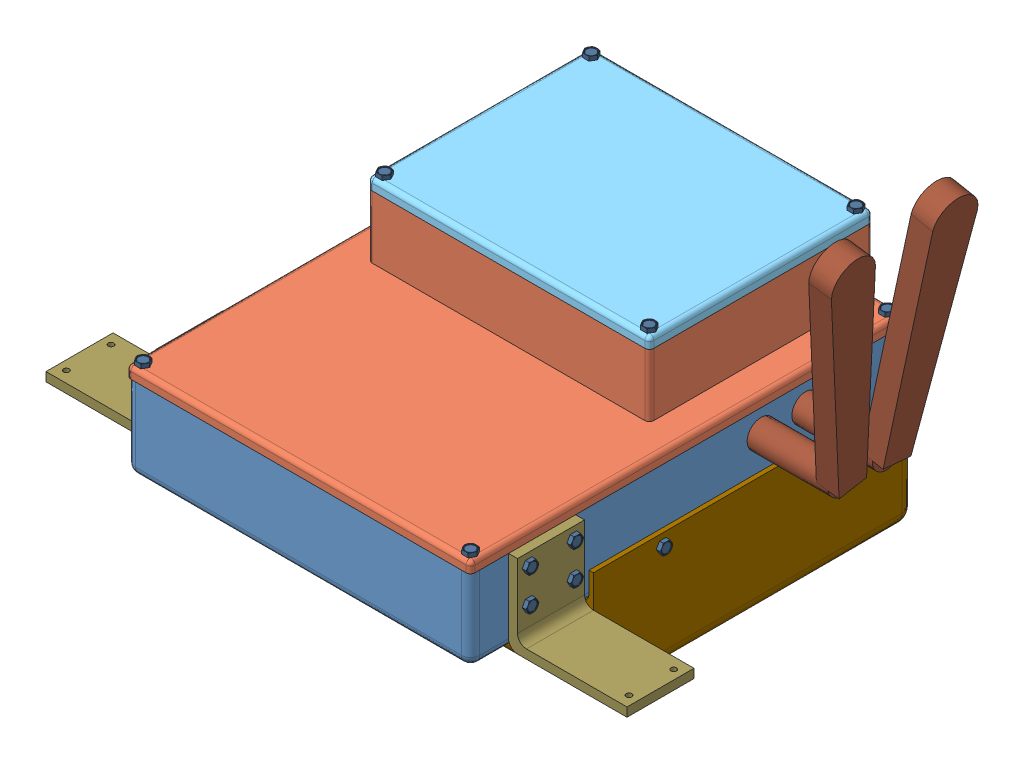
SolidWorks assembly BoxV2, configuration Default. Lengths in mm.
Overall size (339.12 223.08 251.92).
42 component instances, 13 part files, 71 mates.
Components (placement in the parent):
- BoxV2-1: BoxV2 [Default] at (61.0947 94.6993 147.1764) size (262.89 46.99 246.38)
- BoxLidV2-1: BoxLidV2 [Default] at (61.0947 139.1493 147.1764) size (195.58 41.91 246.38)
- ArduinoBoard-1: ArduinoBoard [Default] at (29.0348 145.4993 61.6863) x (-1 0 0) z (0 0 -1) size (81.5 25.4 60)
- Jetson-1: Jetson [Default] at (59.8247 94.6993 172.5764) x (0 0 -1) z (1 0 0) size (170.18 34.29 170.18)
- BoxTopLid-1: BoxTopLid [Default] at (-18.9153 181.0593 23.9864) x (1 0 0) z (0 1 0) size (160.02 127 6.35)
- Power Meter-1: Power Meter [Default] at (-23.9953 69.9343 85.2639) x (0 1 0) z (0 0 -1) size (44.45 25.4 85.72)
- Power Meter-2: Power Meter [Default] at (146.1847 69.9343 85.2639) x (0 -1 0) z (0 0 -1) size (44.45 25.4 85.72)
- Computer Battery-1: Computer Battery [Default] at (59.1897 57.2343 90.0264) size (31.75 34.92 76.2)
- Motor Battery-1: Motor Battery [Default] at (63.6347 69.9343 197.9764) x (0 1 0) z (-1 0 0) size (44.45 57.15 139.7)
- Battery Box-1: Battery Box [Default] at (159.5197 108.6693 23.3514) x (-1 0 0) z (0 -1 0) size (201.93 182.88 66.04)
- #6 Screw-1: #6 Screw [93075A148] at (154.1222 145.4993 265.6039) x (0.866025 0 0.5) z (0 1 0) size (6.35 7.33 15.34)
- #6 Screw-2: #6 Screw [93075A148] at (154.1222 145.4993 28.7489) x (0.866025 0 0.5) z (0 1 0) size (6.35 7.33 15.34)
- #6 Screw-3: #6 Screw [93075A148] at (-31.9328 145.4993 265.6039) x (0.866025 0 0.5) z (0 1 0) size (6.35 7.33 15.34)
- #6 Screw-4: #6 Screw [93075A148] at (-31.9328 145.4993 28.7489) x (0.866025 0 0.5) z (0 1 0) size (6.35 7.33 15.34)
- #6 Screw-5: #6 Screw [93075A148] at (136.3422 187.4093 146.2239) x (0.866025 0 -0.5) z (0 1 0) size (6.35 7.33 15.34)
- #6 Screw-6: #6 Screw [93075A148] at (136.3422 187.4093 28.7489) x (0.866025 0 -0.5) z (0 1 0) size (6.35 7.33 15.34)
- #6 Screw-7: #6 Screw [93075A148] at (-14.1528 187.4093 146.2239) x (0.866025 0 -0.5) z (0 1 0) size (6.35 7.33 15.34)
- #6 Screw-8: #6 Screw [93075A148] at (-14.1528 187.4093 28.7489) x (0.866025 0 -0.5) z (0 1 0) size (6.35 7.33 15.34)
- #6 Screw-9: #6 Screw [93075A148] at (143.0097 102.3193 20.8114) x (-0.866025 -0.5 0) z (0 0 -1) size (6.35 7.33 15.34)
- #6 Screw-10: #6 Screw [93075A148] at (162.0597 102.3193 164.3214) x (0 0.5 -0.866025) z (1 0 0) size (6.35 7.33 15.34)
- #6 Screw-11: #6 Screw [93075A148] at (-39.8703 102.3193 164.3214) x (0 -0.5 0.866025) z (-1 0 0) size (6.35 7.33 15.34)
- #6 Screw-12: #6 Screw [93075A148] at (-20.8203 102.3193 20.8114) x (-0.866025 0.5 0) z (0 0 -1) size (6.35 7.33 15.34)
- Wifi Antenna-1: Wifi Antenna [Default] at (158.8847 126.4493 105.2664) x (0 -0.173648 0.984808) z (0 0.984808 0.173648) size (25.4 76.23 146.62)
- Wifi Antenna-2: Wifi Antenna [Default] at (158.8847 126.4493 79.8664) x (0 0.087156 0.996195) z (0 0.996195 -0.087156) size (25.4 76.23 146.62)
- Mount Angle-1: Mount Angle [Default] at (158.8847 92.1593 210.6764) size (67.31 46.99 38.1)
- Mount Angle-2: Mount Angle [Default] at (-36.6953 92.1593 248.7764) x (-1 0 0) z (0 0 -1) size (67.31 46.99 38.1)
- #6 Screw-13: #6 Screw [93075A148] at (163.9647 132.7993 242.4264) x (0 0.5 -0.866025) z (1 0 0) size (6.35 7.33 15.34)
- #6 Screw-14: #6 Screw [93075A148] at (-41.7753 132.7993 242.4264) x (0 -0.5 0.866025) z (-1 0 0) size (6.35 7.33 15.34)
- #6 Screw-15: #6 Screw [93075A148] at (163.9647 113.7493 242.4264) x (0 0.5 -0.866025) z (1 0 0) size (6.35 7.33 15.34)
- #6 Screw-16: #6 Screw [93075A148] at (163.9647 132.7993 217.0264) x (0 0.5 -0.866025) z (1 0 0) size (6.35 7.33 15.34)
- #6 Screw-17: #6 Screw [93075A148] at (163.9647 113.7493 217.0264) x (0 0.5 -0.866025) z (1 0 0) size (6.35 7.33 15.34)
- #6 Screw-18: #6 Screw [93075A148] at (-41.7753 113.7493 242.4264) x (0 -0.5 0.866025) z (-1 0 0) size (6.35 7.33 15.34)
- #6 Screw-19: #6 Screw [93075A148] at (-41.7753 132.7993 217.0264) x (0 -0.5 0.866025) z (-1 0 0) size (6.35 7.33 15.34)
- #6 Screw-20: #6 Screw [93075A148] at (-41.7753 113.7493 217.0264) x (0 -0.5 0.866025) z (-1 0 0) size (6.35 7.33 15.34)
- #6 Screw Nut-1: #6 Screw Nut [91813A130] at (154.9556 132.7993 242.4264) x (0 0.5 -0.866025) z (0 -0.866025 -0.5) size (7.94 3.39 9.17)
- #6 Screw Nut-2: #6 Screw Nut [91813A130] at (-32.7663 132.7993 242.4264) x (0 1 0) z (0 0 1) size (7.94 3.39 9.17)
- #6 Screw Nut-3: #6 Screw Nut [91813A130] at (154.9556 113.7493 242.4264) x (0 0.5 -0.866025) z (0 -0.866025 -0.5) size (7.94 3.39 9.17)
- #6 Screw Nut-4: #6 Screw Nut [91813A130] at (154.9556 132.7993 217.0264) x (0 0.5 -0.866025) z (0 -0.866025 -0.5) size (7.94 3.39 9.17)
- #6 Screw Nut-5: #6 Screw Nut [91813A130] at (154.9556 113.7493 217.0264) x (0 0.5 -0.866025) z (0 -0.866025 -0.5) size (7.94 3.39 9.17)
- #6 Screw Nut-6: #6 Screw Nut [91813A130] at (-32.7663 113.7493 242.4264) x (0 1 0) z (0 0 1) size (7.94 3.39 9.17)
- #6 Screw Nut-7: #6 Screw Nut [91813A130] at (-32.7663 132.7993 217.0264) x (0 1 0) z (0 0 1) size (7.94 3.39 9.17)
- #6 Screw Nut-8: #6 Screw Nut [91813A130] at (-32.7663 113.7493 217.0264) x (0 1 0) z (0 0 1) size (7.94 3.39 9.17)
Mates (geometry in assembly coordinates):
- Coincident1: coincident anti-aligned: plane of BoxV2-1 through (61.0947 139.1493 147.1764) normal (0 1 0); plane of BoxLidV2-1 through (61.0947 139.1493 147.1764) normal (0 -1 0)
- Coincident9: coincident anti-aligned: plane of BoxV2-1 through (61.0947 94.6993 147.1764) normal (0 1 0); plane of Jetson-1 through (59.8247 94.6993 172.5764) normal (0 -1 0)
- Coincident11: coincident aligned: plane of BoxLidV2-1 through (-36.6953 145.4993 23.9864) normal (-1 0 0); plane of BoxV2-1 through (-36.6953 139.1493 26.5264) normal (-1 0 0)
- Coincident12: coincident aligned: plane of BoxV2-1 through (-34.1553 139.1493 270.3664) normal (0 0 1); plane of BoxLidV2-1 through (-36.6953 145.4993 270.3664) normal (0 0 1)
- Coincident13: coincident anti-aligned: plane of BoxLidV2-1 through (61.0947 181.0593 147.1764) normal (0 1 0); plane of BoxTopLid-1 through (-18.9153 181.0593 23.9864) normal (0 -1 0)
- Concentric2: concentric aligned: cylinder of Jetson-1 through (-18.9153 97.2393 252.5864) axis (0 1 0) radius 2; cylinder of BoxV2-1 through (-18.9153 94.6993 252.5864) axis (0 1 0) radius 2
- Parallel1: parallel: line of Jetson-1 through (-25.2653 97.2393 87.4864) axis (0 0 1); plane of BoxV2-1 through (-34.1553 139.1493 26.5264) normal (1 0 0)
- Concentric3: concentric aligned: cylinder of ArduinoBoard-1 through (64.7848 170.8993 86.6863) axis (0 1 0) radius 1.6; cylinder of BoxLidV2-1 through (64.7848 145.4993 86.6863) axis (0 1 0) radius 1.6
- Parallel2: parallel aligned: plane of ArduinoBoard-1 through (69.7848 170.8993 91.6863) normal (0 0 1); plane of BoxLidV2-1 through (-36.6953 145.4993 26.5264) normal (0 0 1)
- Parallel3: parallel anti-aligned: plane of BoxLidV2-1 through (138.5647 181.0593 150.9864) normal (-1 0 0); plane of ArduinoBoard-1 through (69.7848 170.8993 91.6863) normal (1 0 0)
- Coincident19: coincident anti-aligned: plane of BoxLidV2-1 through (61.0947 145.4993 147.1764) normal (0 1 0); plane of ArduinoBoard-1 through (29.0348 145.4993 61.6863) normal (0 -1 0)
- Coincident20: coincident anti-aligned: plane of BoxV2-1 through (61.0947 92.1593 147.1764) normal (0 -1 0); plane of Motor Battery-1 through (133.4847 92.1593 140.8264) normal (0 1 0)
- Coincident23: coincident anti-aligned: plane of BoxV2-1 through (61.0947 92.1593 147.1764) normal (0 -1 0); plane of Computer Battery-1 through (59.1897 92.1593 90.0264) normal (0 1 0)
- Distance8: distance = 129.54 mm anti-aligned: plane of Motor Battery-1 through (63.6347 69.9343 140.8264) normal (0 0 -1); plane of BoxV2-1 through (-34.1553 139.1493 270.3664) normal (0 0 1)
- Distance9: distance = 25.4 mm aligned: plane of Motor Battery-1 through (133.4847 47.7093 140.8264) normal (1 0 0); plane of BoxV2-1 through (158.8847 139.1493 26.5264) normal (1 0 0)
- Distance12: distance = 12.7 mm anti-aligned: plane of Power Meter-1 through (1.4047 47.7093 128.1264) normal (0 0 1); plane of Motor Battery-1 through (63.6347 69.9343 140.8264) normal (0 0 -1)
- Coincident48: coincident aligned: plane of Computer Battery-1 through (43.3147 92.1593 128.1264) normal (0 0 1); plane of Power Meter-1 through (1.4047 47.7093 128.1264) normal (0 0 1)
- Coincident50: coincident aligned: plane of BoxLidV2-1 through (-36.6953 145.4993 23.9864) normal (0 0 -1); plane of BoxTopLid-1 through (-18.9153 187.4093 23.9864) normal (0 0 -1)
- Coincident51: coincident aligned: plane of BoxLidV2-1 through (141.1047 181.0593 150.9864) normal (1 0 0); plane of BoxTopLid-1 through (141.1047 187.4093 23.9864) normal (1 0 0)
- Coincident52: coincident aligned: plane of Power Meter-2 through (120.7847 92.1593 128.1264) normal (0 0 1); plane of Computer Battery-1 through (43.3147 92.1593 128.1264) normal (0 0 1)
- Distance14: distance = 12.7 mm aligned: plane of BoxV2-1 through (158.8847 139.1493 26.5264) normal (1 0 0); plane of Power Meter-2 through (146.1847 69.9343 85.2639) normal (1 0 0)
- Coincident54: coincident anti-aligned: plane of BoxV2-1 through (61.0947 92.1593 147.1764) normal (0 -1 0); plane of Power Meter-2 through (120.7847 92.1593 128.1264) normal (0 1 0)
- Distance15: distance = 12.7 mm aligned: plane of Power Meter-1 through (-23.9953 69.9343 85.2639) normal (-1 0 0); plane of BoxV2-1 through (-36.6953 139.1493 26.5264) normal (-1 0 0)
- Coincident56: coincident anti-aligned: plane of BoxV2-1 through (61.0947 92.1593 147.1764) normal (0 -1 0); plane of Power Meter-1 through (1.4047 92.1593 128.1264) normal (0 1 0)
- Distance16: distance = 45.72 mm anti-aligned: plane of Power Meter-2 through (120.7847 69.9343 85.2639) normal (-1 0 0); plane of Computer Battery-1 through (75.0647 92.1593 51.9264) normal (1 0 0)
- Coincident64: coincident anti-aligned: plane of BoxLidV2-1 through (61.0947 145.4993 147.1764) normal (0 1 0); plane of #6 Screw-1 through (154.1222 145.4993 259.2539) normal (0 -1 0)
- Concentric4: concentric anti-aligned: cylinder of BoxLidV2-1 through (154.1222 139.1493 265.6039) axis (0 -1 0) radius 1.905; circle of #6 Screw-1
- Coincident65: coincident anti-aligned: plane of BoxTopLid-1 through (-18.9153 187.4093 23.9864) normal (0 1 0); plane of #6 Screw-5 through (130.8429 187.4093 143.0489) normal (0 -1 0)
- Concentric5: concentric anti-aligned: cylinder of BoxTopLid-1 through (136.3422 181.0593 146.2239) axis (0 -1 0) radius 1.905; circle of #6 Screw-5
- Parallel4: parallel anti-aligned: plane of BoxV2-1 through (-34.1553 139.1493 270.3664) normal (0 0 1); plane of #6 Screw-1 through (155.9553 147.8615 262.4289) normal (0 0 -1)
- Parallel5: parallel aligned: plane of BoxLidV2-1 through (-18.9153 181.0593 150.9864) normal (0 0 1); plane of #6 Screw-5 through (134.5091 189.7715 149.3989) normal (0 0 1)
- Coincident68: coincident anti-aligned: plane of Battery Box-1 through (159.5197 45.1693 20.8114) normal (0 0 -1); plane of #6 Screw-9 through (143.0097 108.6693 20.8114) normal (0 0 1)
- Concentric6: concentric aligned: circle of Battery Box-1; circle of #6 Screw-9
- Coincident69: coincident anti-aligned: plane of Battery Box-1 through (162.0597 45.1693 23.3514) normal (1 0 0); plane of #6 Screw-10 through (162.0597 105.4943 169.8206) normal (-1 0 0)
- Concentric7: concentric aligned: cylinder of Battery Box-1 through (162.0597 102.3193 164.3214) axis (1 0 0) radius 1.786; circle of #6 Screw-10
- Coincident70: coincident anti-aligned: plane of Battery Box-1 through (159.5197 45.1693 20.8114) normal (0 0 -1); plane of #6 Screw-12 through (-15.3211 105.4943 20.8114) normal (0 0 1)
- Concentric8: concentric aligned: circle of Battery Box-1; circle of #6 Screw-12
- Coincident71: coincident anti-aligned: plane of Battery Box-1 through (-39.8703 45.1693 23.3514) normal (-1 0 0); plane of #6 Screw-11 through (-39.8703 108.6693 164.3214) normal (1 0 0)
- Concentric9: concentric anti-aligned: cylinder of Battery Box-1 through (162.0597 102.3193 164.3214) axis (1 0 0) radius 1.786; circle of #6 Screw-11
- Parallel6: parallel aligned: plane of Battery Box-1 through (159.5197 108.6693 23.3514) normal (0 1 0); plane of #6 Screw-11 through (-42.2325 105.4943 166.1544) normal (0 1 0)
- Parallel7: parallel aligned: plane of Battery Box-1 through (159.5197 108.6693 23.3514) normal (0 1 0); plane of #6 Screw-12 through (-22.6534 105.4943 18.4492) normal (0 1 0)
- Parallel8: parallel aligned: plane of Battery Box-1 through (159.5197 108.6693 23.3514) normal (0 1 0); plane of #6 Screw-9 through (141.1766 105.4943 18.4492) normal (0 1 0)
- Parallel9: parallel aligned: plane of Battery Box-1 through (159.5197 108.6693 23.3514) normal (0 1 0); plane of #6 Screw-10 through (164.4219 105.4943 162.4883) normal (0 1 0)
- Distance21: distance = 25.4 mm: line of Wifi Antenna-1 through (151.435 126.4493 105.2664) axis (1 0 0); line of Wifi Antenna-2 through (151.435 126.4493 79.8664) axis (1 0 0)
- Coincident73: coincident anti-aligned: plane of BoxV2-1 through (158.8847 139.1493 26.5264) normal (1 0 0); plane of Wifi Antenna-1 through (158.8847 126.4493 105.2664) normal (-1 0 0)
- Coincident75: coincident anti-aligned: plane of BoxV2-1 through (158.8847 139.1493 26.5264) normal (1 0 0); plane of Wifi Antenna-2 through (158.8847 126.4493 79.8664) normal (-1 0 0)
- Distance23: distance = 12.7 mm: line of Wifi Antenna-1 through (151.435 126.4493 105.2664) axis (1 0 0); line of BoxLidV2-1 through (158.8847 139.1493 267.8264) axis (0 0 -1)
- Distance26: distance = 160.02 mm: line of Wifi Antenna-1 through (151.435 126.4493 105.2664) axis (1 0 0); line of BoxV2-1 through (158.8847 139.1493 265.2864) axis (0 -1 0)
- Distance25: distance = 12.7 mm: line of Wifi Antenna-2 through (151.435 126.4493 79.8664) axis (1 0 0); line of BoxLidV2-1 through (158.8847 139.1493 267.8264) axis (0 0 -1)
- Angle1: planar angle = 0.087266 rad anti-aligned: plane of Wifi Antenna-2 through (158.8847 126.4493 79.8664) normal (0 0.087156 0.996195); plane of BoxV2-1 through (-34.1553 139.1493 23.9864) normal (0 0 -1)
- Angle2: planar angle = 0.174533 rad anti-aligned: plane of Wifi Antenna-1 through (158.8847 126.4493 105.2664) normal (0 -0.173648 0.984808); plane of BoxV2-1 through (-34.1553 139.1493 23.9864) normal (0 0 -1)
- Concentric14: concentric anti-aligned: cylinder of BoxV2-1 through (158.8847 102.3193 164.3214) axis (1 0 0) radius 1.905; circle of #6 Screw-11
- Concentric15: concentric aligned: circle of BoxV2-1; circle of #6 Screw-12
- Concentric16: concentric aligned: circle of BoxV2-1; circle of Mount Angle-1
- Coincident77: coincident anti-aligned: plane of BoxV2-1 through (158.8847 139.1493 26.5264) normal (1 0 0); plane of Mount Angle-1 through (158.8847 97.2393 248.7764) normal (-1 0 0)
- Concentric17: concentric aligned: cylinder of BoxV2-1 through (158.8847 132.7993 217.0264) axis (1 0 0) radius 1.905; cylinder of Mount Angle-1 through (163.9647 132.7993 217.0264) axis (1 0 0) radius 1.905
- Coincident78: coincident anti-aligned: plane of BoxV2-1 through (-36.6953 139.1493 26.5264) normal (-1 0 0); plane of Mount Angle-2 through (-36.6953 97.2393 210.6764) normal (1 0 0)
- Concentric18: concentric anti-aligned: cylinder of BoxV2-1 through (158.8847 132.7993 242.4264) axis (1 0 0) radius 1.905; cylinder of Mount Angle-2 through (-41.7753 132.7993 242.4264) axis (-1 0 0) radius 1.905
- Coincident79: coincident anti-aligned: circle of BoxV2-1; cylinder of Mount Angle-2 through (-41.7753 132.7993 217.0264) axis (-1 0 0) radius 1.905
- Coincident80: coincident anti-aligned: plane of Mount Angle-1 through (163.9647 102.3193 248.7764) normal (1 0 0); plane of #6 Screw-13 through (163.9647 135.9743 247.9256) normal (-1 0 0)
- Concentric19: concentric aligned: cylinder of Mount Angle-1 through (163.9647 132.7993 242.4264) axis (1 0 0) radius 1.905; circle of #6 Screw-13
- Parallel10: parallel aligned: plane of Mount Angle-1 through (158.8847 139.1493 248.7764) normal (0 1 0); plane of #6 Screw-13 through (166.3269 135.9743 240.5933) normal (0 1 0)
- Coincident82: coincident anti-aligned: plane of Mount Angle-2 through (-41.7753 102.3193 210.6764) normal (-1 0 0); plane of #6 Screw-14 through (-41.7753 139.1493 242.4264) normal (1 0 0)
- Concentric20: concentric aligned: circle of Mount Angle-2; circle of #6 Screw-14
- Parallel11: parallel aligned: plane of Mount Angle-2 through (-36.6953 139.1493 210.6764) normal (0 1 0); plane of #6 Screw-14 through (-44.1375 135.9743 244.2594) normal (0 1 0)
- Coincident84: coincident anti-aligned: plane of BoxV2-1 through (156.3447 139.1493 26.5264) normal (-1 0 0); plane of #6 Screw Nut-1 through (156.3447 132.7993 247.0091) normal (1 0 0)
- Concentric21: concentric anti-aligned: circle of BoxV2-1; circle of #6 Screw Nut-1
- Parallel12: parallel aligned: plane of Mount Angle-1 through (158.8847 139.1493 248.7764) normal (0 1 0); plane of #6 Screw Nut-1 through (156.3447 136.7681 240.135) normal (0 1 0)
- Coincident86: coincident anti-aligned: plane of BoxV2-1 through (-34.1553 139.1493 26.5264) normal (1 0 0); plane of #6 Screw Nut-2 through (-34.1553 128.8306 240.135) normal (-1 0 0)
- Concentric22: concentric anti-aligned: circle of BoxV2-1; circle of #6 Screw Nut-2
- Parallel13: parallel aligned: plane of BoxV2-1 through (61.0947 139.1493 147.1764) normal (0 1 0); plane of #6 Screw Nut-2 through (-34.1553 136.7681 244.7177) normal (0 1 0)
